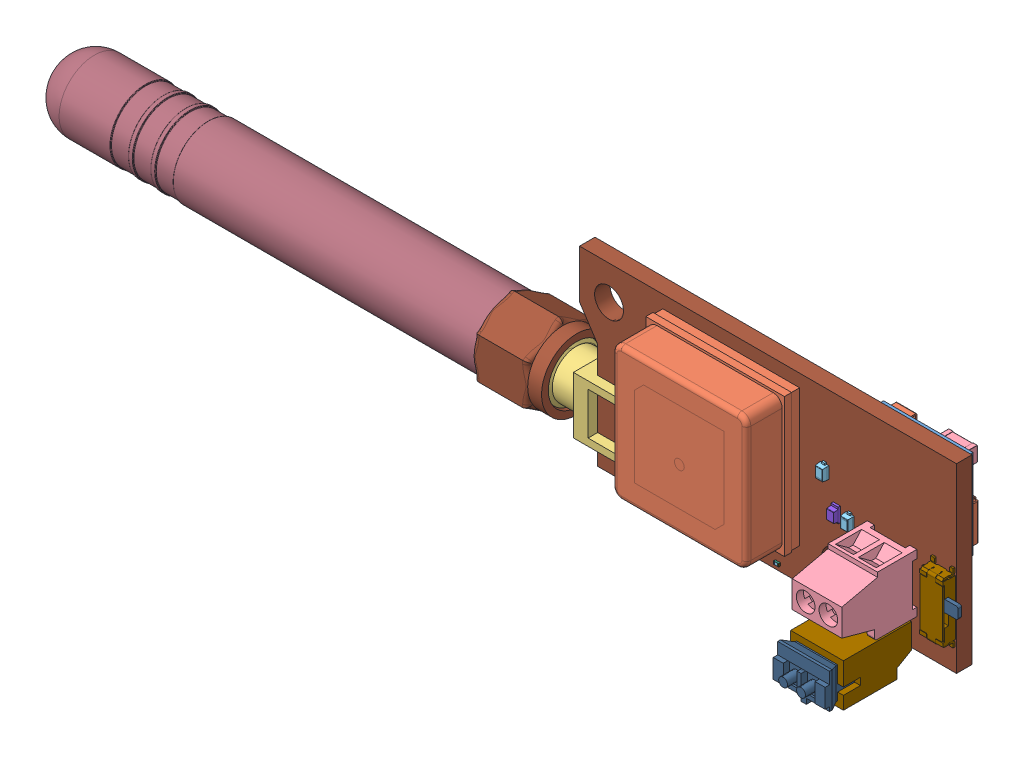
SolidWorks assembly Featherweight GPS, configuration Default. Lengths in mm.
Overall size (103.47 21.82 17.26).
178 component instances, 47 part files, 0 mates.
Components (placement in the parent):
- CYBLE-222014-01 BLE Module_0R0_AP214.step-1: CYBLE-222014-01 BLE Module_0R0_AP214.step [Default] at origin size (10 10 1.79)
  - CYBLE-222005 PCB.step-1: CYBLE-222005 PCB.step [Default] at (28.481 3.6068 0) x (1 0 0) z (0 1 0) size (10 0.5 10)
  - Sheild.step-1: Sheild.step [Default] at (25.7239 -6.0922 -1.49) x (1 0 0) z (0 1 0) size (9.42 1 9.4)
  - 001-96603-A.step-1: 001-96603-A.step [Default] at (33.4749 -3.5332 -0.71) x (0 1 0) z (-1 0 0) size (4.04 0.51 3.87)
  - 2450AT18B100 Antenna 3.2x1.6x0.step-1: 2450AT18B100 Antenna 3.2x1.6x0.step [Default] at (36.0872 2.4305 -1.14) x (1 0 0) z (0 1 0) size (3.2 1.3 1.65)
  - Xtal 1.6x1.0x0.step-1: Xtal 1.6x1.0x0.step [Default] at (36.8746 -2.4839 -0.49) x (1 0 0) z (0 1 0) size (1.6 0.45 1)
  - Xtal 2.5x2.0x0.step-1: Xtal 2.5x2.0x0.step [Default] at (30.2673 -4.1843 -0.495) x (0 1 0) z (-1 0 0) size (2.5 0.51 2)
  - L0603x033(0201).step-1: L0603x033(0201).step [Default] at (30.6421 0.2552 -0.5) x (0 -1 0) z (1 0 0) size (0.6 0.33 0.3)
  - L0603x033(0201).step-2: L0603x033(0201).step [Default] at (30.6471 2.1351 -0.5) x (0 -1 0) z (1 0 0) size (0.6 0.33 0.3)
  - Cap0603x030(0201).step-1: Cap0603x030(0201).step [Default] at (30.3676 1.1604 -0.5) x (1 0 0) z (0 1 0) size (0.6 0.3 0.3)
  - Cap0603x030(0201).step-2: Cap0603x030(0201).step [Default] at (30.3891 -0.6461 -0.5) x (1 0 0) z (0 1 0) size (0.6 0.3 0.3)
  - Cap0603x030(0201).step-3: Cap0603x030(0201).step [Default] at (29.5002 -0.6389 -0.5) x (0 -1 0) z (1 0 0) size (0.6 0.3 0.3)
  - Cap0603x030(0201).step-4: Cap0603x030(0201).step [Default] at (29.5146 -2.1515 -0.5) x (0 -1 0) z (1 0 0) size (0.6 0.3 0.3)
  - Cap0603x030(0201).step-5: Cap0603x030(0201).step [Default] at (30.1454 -2.1371 -0.5) x (0 -1 0) z (1 0 0) size (0.6 0.3 0.3)
  - Cap0603x030(0201).step-6: Cap0603x030(0201).step [Default] at (30.7547 -2.1228 -0.5) x (0 -1 0) z (1 0 0) size (0.6 0.3 0.3)
  - Cap0603x030(0201).step-7: Cap0603x030(0201).step [Default] at (31.9926 -5.9585 -0.5) x (1 0 0) z (0 1 0) size (0.6 0.3 0.3)
  - Cap0603x030(0201).step-8: Cap0603x030(0201).step [Default] at (33.1629 -5.9505 -0.5) x (1 0 0) z (0 1 0) size (0.6 0.3 0.3)
  - Cap0603x030(0201).step-9: Cap0603x030(0201).step [Default] at (34.3088 -5.9554 -0.5) x (1 0 0) z (0 1 0) size (0.6 0.3 0.3)
  - Cap0603x030(0201).step-10: Cap0603x030(0201).step [Default] at (35.4989 -5.9372 -0.5) x (1 0 0) z (0 1 0) size (0.6 0.3 0.3)
  - Cap0603x030(0201).step-11: Cap0603x030(0201).step [Default] at (36.5237 -4.2251 -0.5) x (1 0 0) z (0 1 0) size (0.6 0.3 0.3)
  - Cap0603x030(0201).step-12: Cap0603x030(0201).step [Default] at (36.5155 -3.4775 -0.5) x (1 0 0) z (0 1 0) size (0.6 0.3 0.3)
  - Cap0603x030(0201).step-13: Cap0603x030(0201).step [Default] at (37.4274 -3.7239 -0.5) x (0 -1 0) z (1 0 0) size (0.6 0.3 0.3)
  - Cap0603x030(0201).step-14: Cap0603x030(0201).step [Default] at (36.4416 -5.1698 -0.5) x (0 -1 0) z (1 0 0) size (0.6 0.3 0.3)
  - Cap0603x030(0201).step-15: Cap0603x030(0201).step [Default] at (37.0659 -5.1616 -0.5) x (0 -1 0) z (1 0 0) size (0.6 0.3 0.3)
- CUS-12TB.step-1: CUS-12TB.step [Default] at origin size (5 7.7 1.9)
  - _CUS-12-body.step-1: _CUS-12-body.step [Default] at (37.4289 -10.1846 1.7272) x (0 1 0) z (1 0 0) size (7.7 1.9 3.5)
  - _CUS-12-slider.step-1: _CUS-12-slider.step [Default] at (38.2289 -9.4346 2.9272) x (0 1 0) z (1 0 0) size (1.3 0.4 2.05)
- Antenna.step-1: Antenna.step [Default] at origin size (57.52 9.15 7.94)
  - RSP.step-1: RSP.step [Default] at (-10.2539 -10.8712 -0.3778) x (0 1 0) z (0 0 -1) size (9.15 13.52 7.94)
  - RSP-MA1.step-1: RSP-MA1.step [Default] at (-14.0004 -10.8712 -0.3778) x (0 1 0) z (-1 0 0) size (1.65 1.65 7.62)
  - Antenna_1.step-1: Antenna_1.step [Default] at (-10.2539 -10.8712 -0.3778) x (0 1 0) z (0 0 -1) size (7.9 50 7.9)
- LoRa Module.step-1: LoRa Module.step [Default] at origin size (12.5 14 1.77)
  - PCB.step-1: PCB.step [Default] at (12.3863 -7.4346 0) x (0 -1 0) z (1 0 0) size (11.6 0.6 12.5)
  - Shield.step-1: Shield.step [Default] at (12.3863 -7.4346 -1.76) x (0 -1 0) z (1 0 0) size (11.42 1.16 12.42)
  - Label.step-1: Label.step [Default] at (12.3863 -7.4346 -1.76) x (0 0 -1) z (1 0 0) size (0.01 14 9.3)
- R0402.step-1: R0402.step [Default] at (13.7605 8.0124 0) x (0 -1 0) z (0 0 1) size (1.1 0.5 0.32)
  - R0402_detailed.step-1: R0402_detailed.step [Default] at (7.3529 -0.5851 0) x (-1 0 0) z (0 0 -1) size (1.1 0.5 0.32)
    - Part 6.step-1: Part 6.step [Default] at origin size (0.74 0.5 0.02)
    - Part 5.step-1: Part 5.step [Default] at origin size (1.05 0.5 0.27)
    - Part 4.step-1: Part 4.step [Default] at origin size (0.08 0.38 0.03)
    - Part 3.step-1: Part 3.step [Default] at origin size (0.08 0.38 0.03)
    - Part 2.step-1: Part 2.step [Default] at origin size (0.25 0.5 0.32)
    - Part 1.step-1: Part 1.step [Default] at origin size (0.25 0.5 0.32)
- R0402_1.step-1: R0402_1.step [Default] at (13.7605 8.0124 0) x (0 -1 0) z (0 0 1) size (1.1 0.5 0.32)
  - R0402_detailed_1.step-1: R0402_detailed_1.step [Default] at (13.1501 7.891 0) x (-1 0 0) z (0 0 -1) size (1.1 0.5 0.32)
    - Part 6.step-1: Part 6.step [Default] at origin size (0.74 0.5 0.02)
    - Part 5.step-1: Part 5.step [Default] at origin size (1.05 0.5 0.27)
    - Part 4.step-1: Part 4.step [Default] at origin size (0.08 0.38 0.03)
    - Part 3.step-1: Part 3.step [Default] at origin size (0.08 0.38 0.03)
    - Part 2.step-1: Part 2.step [Default] at origin size (0.25 0.5 0.32)
    - Part 1.step-1: Part 1.step [Default] at origin size (0.25 0.5 0.32)
- R0402_2.step-1: R0402_2.step [Default] at (20.3826 -3.2472 0) x (0 -1 0) z (0 0 -1) size (1.1 0.5 0.32)
  - R0402_detailed_2.step-1: R0402_detailed_2.step [Default] at origin size (1.1 0.5 0.32)
    - Part 6.step-1: Part 6.step [Default] at origin size (0.74 0.5 0.02)
    - Part 5.step-1: Part 5.step [Default] at origin size (1.05 0.5 0.27)
    - Part 4.step-1: Part 4.step [Default] at origin size (0.08 0.38 0.03)
    - Part 3.step-1: Part 3.step [Default] at origin size (0.08 0.38 0.03)
    - Part 2.step-1: Part 2.step [Default] at origin size (0.25 0.5 0.32)
    - Part 1.step-1: Part 1.step [Default] at origin size (0.25 0.5 0.32)
- R0402_3.step-1: R0402_3.step [Default] at (27.402 -5.6852 0) x (0 -1 0) z (0 0 -1) size (1.1 0.5 0.32)
  - R0402_detailed_3.step-1: R0402_detailed_3.step [Default] at origin size (1.1 0.5 0.32)
    - Part 6.step-1: Part 6.step [Default] at origin size (0.74 0.5 0.02)
    - Part 5.step-1: Part 5.step [Default] at origin size (1.05 0.5 0.27)
    - Part 4.step-1: Part 4.step [Default] at origin size (0.08 0.38 0.03)
    - Part 3.step-1: Part 3.step [Default] at origin size (0.08 0.38 0.03)
    - Part 2.step-1: Part 2.step [Default] at origin size (0.25 0.5 0.32)
    - Part 1.step-1: Part 1.step [Default] at origin size (0.25 0.5 0.32)
- R0402_4.step-1: R0402_4.step [Default] at (13.7605 8.0124 0) x (0 -1 0) z (0 0 -1) size (0.5 1.1 0.32)
  - R0402_detailed_4.step-1: R0402_detailed_4.step [Default] at (4.9505 -10.644 0) x (0 1 0) z (0 0 1) size (1.1 0.5 0.32)
    - Part 6.step-1: Part 6.step [Default] at origin size (0.74 0.5 0.02)
    - Part 5.step-1: Part 5.step [Default] at origin size (1.05 0.5 0.27)
    - Part 4.step-1: Part 4.step [Default] at origin size (0.08 0.38 0.03)
    - Part 3.step-1: Part 3.step [Default] at origin size (0.08 0.38 0.03)
    - Part 2.step-1: Part 2.step [Default] at origin size (0.25 0.5 0.32)
    - Part 1.step-1: Part 1.step [Default] at origin size (0.25 0.5 0.32)
- R0402_5.step-1: R0402_5.step [Default] at (19.1771 -2.1738 0) x (0 -1 0) z (0 0 1) size (1.1 0.5 0.32)
  - R0402_detailed_5.step-1: R0402_detailed_5.step [Default] at (13.1345 -7.8704 0) x (-1 0 0) z (0 0 -1) size (1.1 0.5 0.32)
    - Part 6.step-1: Part 6.step [Default] at origin size (0.74 0.5 0.02)
    - Part 5.step-1: Part 5.step [Default] at origin size (1.05 0.5 0.27)
    - Part 4.step-1: Part 4.step [Default] at origin size (0.08 0.38 0.03)
    - Part 3.step-1: Part 3.step [Default] at origin size (0.08 0.38 0.03)
    - Part 2.step-1: Part 2.step [Default] at origin size (0.25 0.5 0.32)
    - Part 1.step-1: Part 1.step [Default] at origin size (0.25 0.5 0.32)
- R0402_6.step-1: R0402_6.step [Default] at (2.0397 21.115 0) x (0 -1 0) z (0 0 1) size (0.5 1.1 0.32)
  - R0402_detailed_6.step-1: R0402_detailed_6.step [Default] at (36.368 12.1316 0) x (0 1 0) z (0 0 -1) size (1.1 0.5 0.32)
    - Part 6.step-1: Part 6.step [Default] at origin size (0.74 0.5 0.02)
    - Part 5.step-1: Part 5.step [Default] at origin size (1.05 0.5 0.27)
    - Part 4.step-1: Part 4.step [Default] at origin size (0.08 0.38 0.03)
    - Part 3.step-1: Part 3.step [Default] at origin size (0.08 0.38 0.03)
    - Part 2.step-1: Part 2.step [Default] at origin size (0.25 0.5 0.32)
    - Part 1.step-1: Part 1.step [Default] at origin size (0.25 0.5 0.32)
- R0402_7.step-1: R0402_7.step [Default] at (2.0397 21.115 0) x (0 -1 0) z (0 0 1) size (1.1 0.5 0.32)
  - R0402_detailed_7.step-1: R0402_detailed_7.step [Default] at (36.4067 10.326 0) x (-1 0 0) z (0 0 -1) size (1.1 0.5 0.32)
    - Part 6.step-1: Part 6.step [Default] at origin size (0.74 0.5 0.02)
    - Part 5.step-1: Part 5.step [Default] at origin size (1.05 0.5 0.27)
    - Part 4.step-1: Part 4.step [Default] at origin size (0.08 0.38 0.03)
    - Part 3.step-1: Part 3.step [Default] at origin size (0.08 0.38 0.03)
    - Part 2.step-1: Part 2.step [Default] at origin size (0.25 0.5 0.32)
    - Part 1.step-1: Part 1.step [Default] at origin size (0.25 0.5 0.32)
- R0201.step-1: R0201.step [Default] at (10.521 -19.9765 0) size (0.6 0.3 0.23)
  - R0201_detailed.step-1: R0201_detailed.step [Default] at (2.451 4.5887 1.7272) size (0.6 0.3 0.23)
    - Part 6_1.step-1: Part 6_1.step [Default] at origin size (0.34 0.3 0.02)
    - Part 5_1.step-1: Part 5_1.step [Default] at origin size (0.55 0.3 0.18)
    - Part 4_1.step-1: Part 4_1.step [Default] at origin size (0.03 0.2 0.03)
    - Part 3_1.step-1: Part 3_1.step [Default] at origin size (0.03 0.2 0.03)
    - Part 2_1.step-1: Part 2_1.step [Default] at origin size (0.15 0.3 0.23)
    - Part 1_1.step-1: Part 1_1.step [Default] at origin size (0.15 0.3 0.23)
- R0201_1.step-1: R0201_1.step [Default] at (10.521 -19.9765 0) size (0.3 0.6 0.23)
  - R0201_detailed_1.step-1: R0201_detailed_1.step [Default] at (-6.6471 16.1051 1.7272) x (0 -1 0) z (0 0 1) size (0.6 0.3 0.23)
    - Part 6_1.step-1: Part 6_1.step [Default] at origin size (0.34 0.3 0.02)
    - Part 5_1.step-1: Part 5_1.step [Default] at origin size (0.55 0.3 0.18)
    - Part 4_1.step-1: Part 4_1.step [Default] at origin size (0.03 0.2 0.03)
    - Part 3_1.step-1: Part 3_1.step [Default] at origin size (0.03 0.2 0.03)
    - Part 2_1.step-1: Part 2_1.step [Default] at origin size (0.15 0.3 0.23)
    - Part 1_1.step-1: Part 1_1.step [Default] at origin size (0.15 0.3 0.23)
- R0201_2.step-1: R0201_2.step [Default] at (10.521 -19.9765 0) size (0.6 0.3 0.23)
  - R0201_detailed_2.step-1: R0201_detailed_2.step [Default] at (4.7243 4.6218 1.7272) size (0.6 0.3 0.23)
    - Part 6_1.step-1: Part 6_1.step [Default] at origin size (0.34 0.3 0.02)
    - Part 5_1.step-1: Part 5_1.step [Default] at origin size (0.55 0.3 0.18)
    - Part 4_1.step-1: Part 4_1.step [Default] at origin size (0.03 0.2 0.03)
    - Part 3_1.step-1: Part 3_1.step [Default] at origin size (0.03 0.2 0.03)
    - Part 2_1.step-1: Part 2_1.step [Default] at origin size (0.15 0.3 0.23)
    - Part 1_1.step-1: Part 1_1.step [Default] at origin size (0.15 0.3 0.23)
- R0201_3.step-1: R0201_3.step [Default] at (10.521 -19.9765 0) size (0.6 0.3 0.23)
  - R0201_detailed_3.step-1: R0201_detailed_3.step [Default] at (8.8191 4.6452 2.1631) size (0.6 0.3 0.23)
    - Part 6_1.step-1: Part 6_1.step [Default] at origin size (0.34 0.3 0.02)
    - Part 5_1.step-1: Part 5_1.step [Default] at origin size (0.55 0.3 0.18)
    - Part 4_1.step-1: Part 4_1.step [Default] at origin size (0.03 0.2 0.03)
    - Part 3_1.step-1: Part 3_1.step [Default] at origin size (0.03 0.2 0.03)
    - Part 2_1.step-1: Part 2_1.step [Default] at origin size (0.15 0.3 0.23)
    - Part 1_1.step-1: Part 1_1.step [Default] at origin size (0.15 0.3 0.23)
- C0402_035.step-1: C0402_035.step [Default] at (20.9649 -18.2521 -2.6622) x (0 -1 0) z (0 0 1) size (1 0.5 0.35)
  - C0402_035_1.step-1: C0402_035_1.step [Default] at (-10.5375 -0.7734 2.3137) size (1 0.5 0.35)
    - Part 3_3.step-1: Part 3_3.step [Default] at origin size (0.85 0.49 0.35)
    - Part 2_3.step-1: Part 2_3.step [Default] at origin size (0.15 0.5 0.35)
    - Part 1_3.step-1: Part 1_3.step [Default] at origin size (0.15 0.5 0.35)
- C0805_085.step-1: C0805_085.step [Default] at origin size (2 1.25 0.85)
  - C0805_085_1.step-1: C0805_085_1.step [Default] at (24.8156 -7.8144 0.015) x (1 0 0) z (0 0 -1) size (2 1.25 0.85)
    - Part 3_2.step-1: Part 3_2.step [Default] at origin size (1.8 1.22 0.82)
    - Part 2_2.step-1: Part 2_2.step [Default] at origin size (0.2 1.25 0.85)
    - Part 1_2.step-1: Part 1_2.step [Default] at origin size (0.2 1.25 0.85)
- C0402_035_2.step-1: C0402_035_2.step [Default] at (22.9247 6.0446 -2.6622) x (0 -1 0) z (0 0 1) size (0.5 1 0.35)
  - C0402_035_3.step-1: C0402_035_3.step [Default] at (3.9591 1.9269 2.3137) x (0 -1 0) z (0 0 1) size (1 0.5 0.35)
    - Part 3_3.step-1: Part 3_3.step [Default] at origin size (0.85 0.49 0.35)
    - Part 2_3.step-1: Part 2_3.step [Default] at origin size (0.15 0.5 0.35)
    - Part 1_3.step-1: Part 1_3.step [Default] at origin size (0.15 0.5 0.35)
- C0603_060.step-1: C0603_060.step [Default] at origin size (1.6 0.8 0.6)
  - C0603_060_1.step-1: C0603_060_1.step [Default] at (16.2684 1.683 -0.585) size (1.6 0.8 0.6)
    - Part 3_4.step-1: Part 3_4.step [Default] at origin size (1.4 0.77 0.57)
    - Part 2_4.step-1: Part 2_4.step [Default] at origin size (0.2 0.8 0.6)
    - Part 1_4.step-1: Part 1_4.step [Default] at origin size (0.2 0.8 0.6)
- C0603_060_2.step-1: C0603_060_2.step [Default] at (14.955 6.5211 0) size (0.8 1.6 0.6)
  - C0603_060_3.step-1: C0603_060_3.step [Default] at (6.6336 -14.5529 -0.585) x (0 1 0) z (0 0 1) size (1.6 0.8 0.6)
    - Part 3_4.step-1: Part 3_4.step [Default] at origin size (1.4 0.77 0.57)
    - Part 2_4.step-1: Part 2_4.step [Default] at origin size (0.2 0.8 0.6)
    - Part 1_4.step-1: Part 1_4.step [Default] at origin size (0.2 0.8 0.6)
- C0603_060_4.step-1: C0603_060_4.step [Default] at (20.7805 6.2602 0) size (0.8 1.6 0.6)
  - C0603_060_5.step-1: C0603_060_5.step [Default] at (1.3279 -7.2606 -0.585) x (0 1 0) z (0 0 1) size (1.6 0.8 0.6)
    - Part 3_4.step-1: Part 3_4.step [Default] at origin size (1.4 0.77 0.57)
    - Part 2_4.step-1: Part 2_4.step [Default] at origin size (0.2 0.8 0.6)
    - Part 1_4.step-1: Part 1_4.step [Default] at origin size (0.2 0.8 0.6)
- C0603_060_6.step-1: C0603_060_6.step [Default] at (22.6933 5.6516 0) size (1.6 0.8 0.6)
  - C0603_060_7.step-1: C0603_060_7.step [Default] at (2.6007 -7.3901 -0.585) size (1.6 0.8 0.6)
    - Part 3_4.step-1: Part 3_4.step [Default] at origin size (1.4 0.77 0.57)
    - Part 2_4.step-1: Part 2_4.step [Default] at origin size (0.2 0.8 0.6)
    - Part 1_4.step-1: Part 1_4.step [Default] at origin size (0.2 0.8 0.6)
- SAM-MQ8-0-10.step-1: SAM-MQ8-0-10.step [Default] at (21.3152 -12.9078 1.7272) x (0 1 0) z (0 0 1) size (15.5 15.5 5.8)
- SAMTEC_SMA-J-P-H-ST-EM1.step-1: SAMTEC_SMA-J-P-H-ST-EM1.step [Default] at (-1.27 -10.8712 0.3972) x (0 1 0) z (-1 0 0) size (6.35 6.35 13.33)
- Wire Terminal 2 Pin.step-1: Wire Terminal 2 Pin.step [Default] at (31.6601 -6.708 4.7272) x (-1 0 0) z (0 1 0) size (5.54 11.8 6.5)
- SOD-523.step-1: SOD-523.step [Default] at (24.148 -4.1736 1.7272) x (0.000005 1 0) z (0 0 1) size (1.7 0.9 0.7)
- SOD-523.step-2: SOD-523.step [Default] at (26.9756 -7.6478 1.7272) x (0 -1 0) z (0 0 1) size (1.7 0.9 0.7)
- SOT23-5.step-1: SOT23-5.step [Default] at (24.6866 -4.1964 0.0078) x (1 0 0) z (0 0 -1) size (2.84 3.01 1.19)
- SOT-666.step-1: SOT-666.step [Default] at (25.0636 0.4873 0) x (0 -1 0) z (0 0 -1) size (1.59 1.6 0.6)
- 0603.step-1: 0603.step [Default] at (25.4805 -7.5846 1.8523) x (0.000073 1 0) z (1 -0.000073 0) size (1.61 0.75 0.8)
- 0603.step-2: 0603.step [Default] at (6.4404 -14.9151 1.8523) x (0 -1 0) z (-1 0 0) size (1.61 0.75 0.8)
- User Library-S2B.step-1: User Library-S2B.step [Default] at (23.9079 -19.208 1.1713) x (-1 0 0) z (0 0 1) size (5.9 8.2 7.6)
- User Library-PHR-2.step-1: User Library-PHR-2.step [Default] at (33.9079 -12.933 8.6963) x (1 0 0) z (0 0 -1) size (5.8 4.5 7.64)
- GPS Tracker.step-1: GPS Tracker.step [Default] at origin size (42.16 20.32 1.73)
